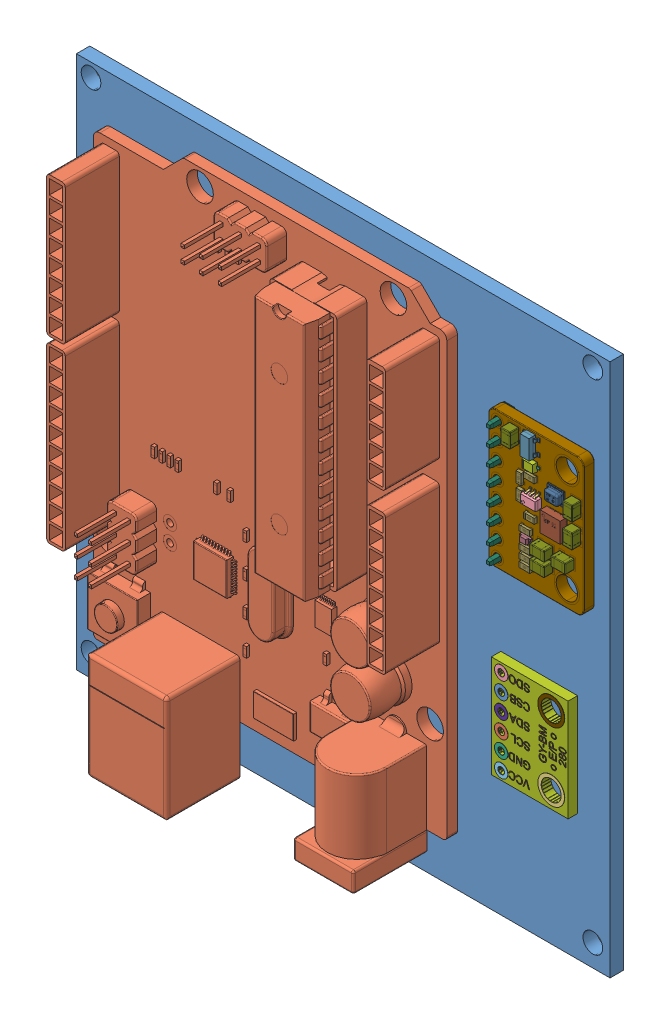
SolidWorks assembly OBC_4, configuration Default. Lengths in mm.
Overall size (80 80.42 20.96).
63 component instances, 29 part files, 0 mates.
Components (placement in the parent):
- Stack_plane_1-1: Stack_plane_1 [Default] at (29.9812 39.7784 61.6823) size (80 80 2)
- arduino uno-1: arduino uno [Default] at (20.6017 39.8567 63.272) x (0 1 0) z (1 0 0) size (76.5 14.6 53)
- GY-91.STEP-1: GY-91.STEP [Default] at (57.713 76.0128 56.2619) x (1 0 0) z (0 -1 0) size (18.43 11.56 29.61)
  - TSSOP-6.STEP-1: TSSOP-6.STEP [Default] at (2.8163 9.9451 17.8096) x (-1 0 0) z (0 1 0) size (2.25 2.25 1.11)
    - User Library-TSSOP-6 (SOT-23-6 PITCH 0.65)_pin_TSSOP_tssop6_1.STEP-1: User Library-TSSOP-6 (SOT-23-6 PITCH 0.65)_pin_TSSOP_tssop6_1.STEP [Default] at (0.65 0.675 0) x (-1 0 0) z (0 1 0) size (0.3 0.82 0.45)
    - User Library-TSSOP-6 (SOT-23-6 PITCH 0.65)_pin_TSSOP_tssop6_1.STEP-2: User Library-TSSOP-6 (SOT-23-6 PITCH 0.65)_pin_TSSOP_tssop6_1.STEP [Default] at (0.65 -0.675 0) x (1 0 0) z (0 -1 0) size (0.3 0.82 0.45)
    - User Library-TSSOP-6 (SOT-23-6 PITCH 0.65)_pin_TSSOP_tssop6_1.STEP-3: User Library-TSSOP-6 (SOT-23-6 PITCH 0.65)_pin_TSSOP_tssop6_1.STEP [Default] at (-0.65 -0.675 0) x (1 0 0) z (0 -1 0) size (0.3 0.82 0.45)
    - User Library-TSSOP-6 (SOT-23-6 PITCH 0.65)_pin_TSSOP_tssop6_1.STEP-4: User Library-TSSOP-6 (SOT-23-6 PITCH 0.65)_pin_TSSOP_tssop6_1.STEP [Default] at (0 0.675 0) x (-1 0 0) z (0 1 0) size (0.3 0.82 0.45)
    - User Library-TSSOP-6 (SOT-23-6 PITCH 0.65)_pin_TSSOP_tssop6_1.STEP-5: User Library-TSSOP-6 (SOT-23-6 PITCH 0.65)_pin_TSSOP_tssop6_1.STEP [Default] at (-0.65 0.675 0) x (-1 0 0) z (0 1 0) size (0.3 0.82 0.45)
    - User Library-TSSOP-6 (SOT-23-6 PITCH 0.65)_pin_TSSOP_tssop6_1.STEP-6: User Library-TSSOP-6 (SOT-23-6 PITCH 0.65)_pin_TSSOP_tssop6_1.STEP [Default] at (0 -0.675 0) x (1 0 0) z (0 -1 0) size (0.3 0.82 0.45)
    - User Library-TSSOP-6 (SOT-23-6 PITCH 0.65)_body_TSSOP-6_TSSOP5_1.STEP-1: User Library-TSSOP-6 (SOT-23-6 PITCH 0.65)_body_TSSOP-6_TSSOP5_1.STEP [Default] at origin size (2.25 1.35 1)
  - Diode.STEP-1: Diode.STEP [Default] at (2.3136 9.1851 13.5607) x (0 0 1) z (0 1 0) size (1.25 2.5 0.7)
    - User Library-SMini2-F5-B_K.STEP-1: User Library-SMini2-F5-B_K.STEP [Default] at origin size (0.5 0.55 0.13)
    - User Library-SMini2-F5-B_A.STEP-1: User Library-SMini2-F5-B_A.STEP [Default] at origin size (0.35 0.55 0.13)
    - User Library-SMini2-F5-B_Diode.STEP-1: User Library-SMini2-F5-B_Diode.STEP [Default] at origin size (1.25 1.7 0.69)
    - User Library-SMini2-F5-B_Marker.STEP-1: User Library-SMini2-F5-B_Marker.STEP [Default] at origin size (1.13 0.07 0.01)
  - gy-91.STEP-1: gy-91.STEP [Default] at (-4.1995 7.585 9.2186) size (14.3 1.6 20.5)
  - BMP280___ _________.STEP-1: BMP280___ _________.STEP [Default] at (7.282 9.2051 14.714) x (-1 0 0) z (0 -1 0) size (2.5 2 0.97)
  - MPU9250.STEP-1: MPU9250.STEP [Default] at (6.0967 9.235 19.3741) x (-1 0 0) z (0 0 -1) size (3.02 1.05 3.02)
  - Res0603.STEP-1: Res0603.STEP [Default] at (0.7709 9.4101 18.2393) x (0 0 1) z (-1 0 0) size (1.6 0.45 0.8)
  - Res0603.STEP-2: Res0603.STEP [Default] at (0.7648 9.4101 15.9917) x (0 0 -1) z (1 0 0) size (1.6 0.45 0.8)
  - Res0603.STEP-3: Res0603.STEP [Default] at (2.312 9.4101 20.4364) size (1.6 0.45 0.8)
  - Res0603.STEP-4: Res0603.STEP [Default] at (1.6231 9.4101 26.0002) size (1.6 0.45 0.8)
  - Res0603.STEP-5: Res0603.STEP [Default] at (1.6278 9.4101 22.3827) size (1.6 0.45 0.8)
  - Res0603.STEP-6: Res0603.STEP [Default] at (2.2995 9.4101 15.1771) size (1.6 0.45 0.8)
  - Res0603.STEP-7: Res0603.STEP [Default] at (1.6136 9.4101 24.8159) size (1.6 0.45 0.8)
  - Res0603.STEP-8: Res0603.STEP [Default] at (1.6314 9.4101 27.1438) size (1.6 0.45 0.8)
  - LED0603.STEP-1: LED0603.STEP [Default] at (2.2297 9.1803 23.5734) x (0 0 1) z (0 1 0) size (0.72 1.65 0.68)
  - LDO SOT23.STEP-1: LDO SOT23.STEP [Default] at (2.3141 9.7351 10.8967) x (0 0 1) z (-1 0 0) size (3 1.1 2.5)
  - MalePinHeader.STEP-1: MalePinHeader.STEP [Default] at (-4.1268 5.0451 16.9269) size (2.54 11.54 2.54)
  - MalePinHeader.STEP-2: MalePinHeader.STEP [Default] at (-4.1071 5.0451 9.3011) size (2.54 11.54 2.54)
  - MalePinHeader.STEP-3: MalePinHeader.STEP [Default] at (-4.1137 5.0451 14.3787) size (2.54 11.54 2.54)
  - MalePinHeader.STEP-4: MalePinHeader.STEP [Default] at (-4.1149 5.0451 27.0667) size (2.54 11.54 2.54)
  - MalePinHeader.STEP-5: MalePinHeader.STEP [Default] at (-4.1277 5.0451 11.82) size (2.54 11.54 2.54)
  - MalePinHeader.STEP-6: MalePinHeader.STEP [Default] at (-4.1157 5.0451 24.5674) size (2.54 11.54 2.54)
  - MalePinHeader.STEP-7: MalePinHeader.STEP [Default] at (-4.1188 5.0451 22.0085) size (2.54 11.54 2.54)
  - MalePinHeader.STEP-8: MalePinHeader.STEP [Default] at (-4.1228 5.0451 19.4816) size (2.54 11.54 2.54)
  - Cap 0805.STEP-1: Cap 0805.STEP [Default] at (52.5692 21.2292 -81.079) x (0 0 -1) z (-1 0 0) size (2.29 1.46 1.49)
  - Cap 0805.STEP-2: Cap 0805.STEP [Default] at (101.2177 21.2292 66.9567) x (1 0 0) z (0 0 -1) size (2.29 1.46 1.49)
  - Cap 0805.STEP-3: Cap 0805.STEP [Default] at (43.25 21.2292 -85.9252) x (0 0 -1) z (-1 0 0) size (2.29 1.46 1.49)
  - Cap 0805.STEP-4: Cap 0805.STEP [Default] at (104.4136 21.2292 66.9514) x (1 0 0) z (0 0 -1) size (2.29 1.46 1.49)
  - Cap 0805.STEP-5: Cap 0805.STEP [Default] at (52.531 21.2292 -77.4673) x (0 0 -1) z (-1 0 0) size (2.29 1.46 1.49)
  - Cap 0805.STEP-6: Cap 0805.STEP [Default] at (101.2189 21.2292 68.9637) x (1 0 0) z (0 0 -1) size (2.29 1.46 1.49)
- P280, 6-PIN-Version v4.step-1: P280, 6-PIN-Version v4.step [Default] at (59.3565 26.3459 65.0982) x (0 1 0) z (0 0 -1) size (15.3 11.5 2.52)
  - PCB.step-1: PCB.step [Default] at origin size (15.3 11.5 1.62)
    - Komponente1.step-1: Komponente1.step [Default] at origin size (2 2 1.62)
    - Komponente2.step-1: Komponente2.step [Default] at origin size (4 4 1.62)
    - Komponente3.step-1: Komponente3.step [Default] at origin size (2 2 1.62)
    - Komponente4.step-1: Komponente4.step [Default] at origin size (2 2 1.62)
    - Komponente5.step-1: Komponente5.step [Default] at origin size (4 4 1.62)
    - Komponente6.step-1: Komponente6.step [Default] at origin size (2 2 1.62)
    - Komponente7.step-1: Komponente7.step [Default] at origin size (2 2 1.62)
    - Komponente8.step-1: Komponente8.step [Default] at origin size (2 2 1.62)
    - PCB-0.step-1: PCB-0.step [Default] at origin size (15.3 11.5 1.55)
  - Bauteile.step-1: Bauteile.step [Default] at origin size (8.8 7.18 0.94)
    - C0603.step-1: C0603.step [Default] at (9.1998 8.6998 1.5493) x (0 -1 0) z (0 0 -1) size (0.8 1.6 0.6)
    - R0603.step-1: R0603.step [Default] at (5.9383 -10.4268 1.548) x (-1 0 0) z (0 0 -1) size (0.8 1.6 0.3)
    - R0603.step-2: R0603.step [Default] at (1.9383 -10.4268 1.548) x (-1 0 0) z (0 0 -1) size (0.8 1.6 0.3)
    - R0603.step-3: R0603.step [Default] at (3.9383 -10.4268 1.548) x (-1 0 0) z (0 0 -1) size (0.8 1.6 0.3)
    - C0603.step-2: C0603.step [Default] at (-0.062 -10.4268 1.5473) x (-1 0 0) z (0 0 -1) size (0.8 1.6 0.6)
    - BME280.step-1: BME280.step [Default] at (2.5 12.9 -0.0401) x (-1 0 0) z (0 0 1) size (2.51 2.5 0.93)
    - R0603.step-4: R0603.step [Default] at (7.9383 -10.4268 1.548) x (-1 0 0) z (0 0 -1) size (0.8 1.6 0.3)
  - Beschriftung.step-1: Beschriftung.step [Default] at origin size (13.63 8.62 0.01)
